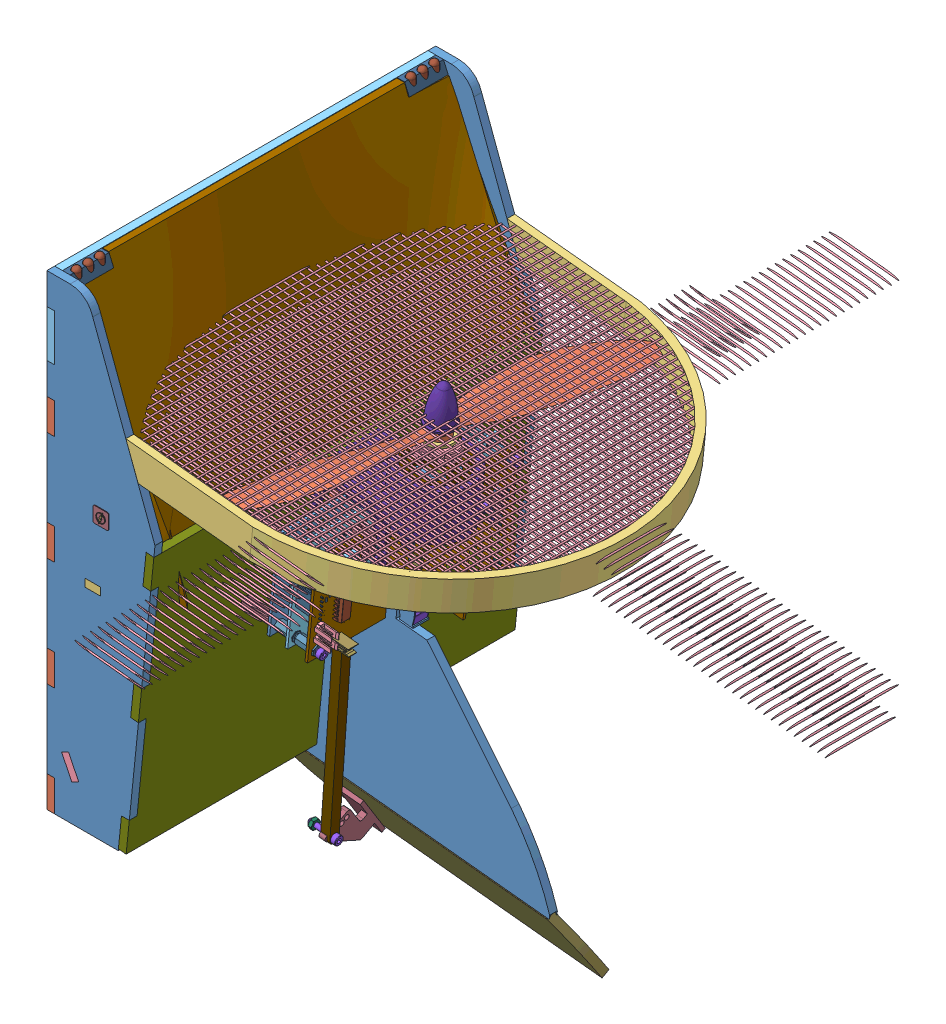
SolidWorks assembly AssTotaleSimu2, configuration Défaut. Lengths in mm.
Overall size (253.25 382.9 251.6).
1779 component instances, 238 part files, 11 mates.
Components (placement in the parent):
- AssStructSimu-1: AssStructSimu [Défaut] at (-125.7658 -1.8483 624.6548) x (1 0 0) z (0 0 -1) size (253.25 324.59 251.6)
  - AssBase-1: AssBase [Défaut] at (36.5482 -71.0398 34.0612) size (86.08 302.3 251.6)
    - AssD-1: AssD [Défaut] at (39.0992 31.0201 8.5) size (69.5 300 22)
      - P1-1: P1 [Défaut] at (-95.5819 194.6656 377.5) size (69.5 300 5)
      - P5-1: P5 [Défaut] at (-100.5819 -35.3344 360.5) x (0 1 0) z (1 0 0) size (230 22 5)
    - AssG-1: AssG [Défaut] at (39.0992 31.0201 -236.5) size (69.5 300 22)
      - P1-1: P1 [Défaut] at (-95.5819 194.6656 377.5) size (69.5 300 5)
      - P5-1: P5 [Défaut] at (-95.5819 -35.3344 399.5) x (0 1 0) z (-1 0 0) size (230 22 5)
    - P7-1: P7 [Défaut] at (-1.4828 89.6857 370.5) x (0 0 -1) z (0 -1 0) size (250 54.5 5)
    - P4-1: P4 [Défaut] at (-63.2363 165.9323 386) x (0 0 -1) z (0.898794 -0.438371 0) size (250 60.5 66.27)
    - P3-1: P3 [Défaut] at (-56.4828 -74.3143 146) x (0 0 1) z (-1 0 0) size (250 70 5)
    - P4b-1: P4b [Défaut] at (-58.7423 163.7404 190) x (0 0 1) z (0.438371 0.898794 0) size (152 56 2)
    - battery-1: battery [Défaut] at (-39.0156 204.1861 197.5) x (0 0 1) z (0.898794 -0.438371 0) size (137 43 30)
    - socket head cap screw 4762_din-1: socket head cap screw 4762_din [EN ISO 4762 M3 x 10 - 10N] at (-27.7008 145.2627 193) x (0.438371 0.898794 0) z (0 0 -1) size (13 5.5 5.5)
    - socket head cap screw 4762_din-2: socket head cap screw 4762_din [EN ISO 4762 M3 x 10 - 10N] at (-27.7008 145.2627 339) x (0.438371 0.898794 0) z (-0.791285 0.385936 -0.474259) size (13 5.5 5.5)
    - socket head cap screw 4762_din-3: socket head cap screw 4762_din [EN ISO 4762 M3 x 10 - 10N] at (-42.0815 152.2766 339) x (0.438371 0.898794 0) z (-0.001489 0.000726 -0.999999) size (13 5.5 5.5)
    - socket head cap screw 4762_din-4: socket head cap screw 4762_din [EN ISO 4762 M3 x 10 - 10N] at (-42.0815 152.2766 193) x (0.438371 0.898794 0) z (-0.031331 0.015281 -0.999392) size (13 5.5 5.5)
    - P11-1: P11 [Défaut] at (-57.5734 -73.9703 146.7843) x (0.005072 0 0.999987) z (0.006197 0.999981 -0.000031) size (240 65 164)
    - AssPhare-1: AssPhare [Défaut] at (-52.8518 -67.6977 411) x (0 1 0) z (0 0 -1) size (35.8 8 25)
      - piece_led-1: piece_led [Défaut] at (-6.6166 -3.631 25) size (7 8 25)
      - LED 5mm-1: LED 5mm [Valor predeterminado] at (-0.1166 0.369 30) x (0 0 1) z (-1 0 0) size (10.06 6 40.8)
      - LED 5mm-2: LED 5mm [Valor predeterminado] at (-0.1166 0.369 37.5) x (0 0 1) z (-1 0 0) size (10.06 6 40.8)
      - LED 5mm-3: LED 5mm [Valor predeterminado] at (-0.1166 0.369 45) x (0 0 1) z (-1 0 0) size (10.06 6 40.8)
    - AssPhare-2: AssPhare [Défaut] at (-52.8518 -67.6977 196) x (0 1 0) z (0 0 -1) size (35.8 8 25)
      - piece_led-1: piece_led [Défaut] at (-6.6166 -3.631 25) size (7 8 25)
      - LED 5mm-1: LED 5mm [Valor predeterminado] at (-0.1166 0.369 30) x (0 0 1) z (-1 0 0) size (10.06 6 40.8)
      - LED 5mm-2: LED 5mm [Valor predeterminado] at (-0.1166 0.369 37.5) x (0 0 1) z (-1 0 0) size (10.06 6 40.8)
      - LED 5mm-3: LED 5mm [Valor predeterminado] at (-0.1166 0.369 45) x (0 0 1) z (-1 0 0) size (10.06 6 40.8)
    - AssLogo-1: AssLogo [Défaut] at (-27.8835 45.1673 148.1054) x (-1 0 0) z (0 0 -1) size (10 10 0.8)
      - logo1-1: logo1 [Défaut] at (-6.5271 -4.4734 6.5054) size (5.8 7.71 0.4)
      - logo2-1: logo2 [Défaut] at (-6.4007 -4.4815 7.1054) size (10 10 0.4)
    - AssLogo-2: AssLogo [Défaut] at (-25.082 45.1673 383.8946) size (10 10 0.8)
      - logo1-1: logo1 [Défaut] at (-6.5271 -4.4734 6.5054) size (5.8 7.71 0.4)
      - logo2-1: logo2 [Défaut] at (-6.4007 -4.4815 7.1054) size (10 10 0.4)
    - support2-1: support2 [Défaut] at (-61.5648 191.7124 276) x (-0.017452 -0.999848 0) z (0.999848 -0.017452 0) size (75 20 10)
    - socket head cap screw 4762_din-5: socket head cap screw 4762_din [EN ISO 4762 M3 x 5 - 5N] at (-61.652 186.7132 269.3333) x (0.999848 -0.017452 0) z (-0.002158 -0.123615 0.992328) size (8 5.5 5.5)
    - socket head cap screw 4762_din-6: socket head cap screw 4762_din [EN ISO 4762 M3 x 5 - 5N] at (-61.652 186.7132 262.6667) x (0.999848 -0.017452 0) z (0 0 1) size (8 5.5 5.5)
    - socket head cap screw 4762_din-7: socket head cap screw 4762_din [EN ISO 4762 M3 x 25 - 18N] at (-55.2963 121.0922 253) x (0 0 1) z (-1 0 0) size (28 5.5 5.5)
    - hex nut style 1 gradeab_din-1: hex nut style 1 gradeab_din [Hexagon Nut ISO 4032 - M3 - W - N] at (-55.2963 121.0922 276) x (-0.923728 -0.383049 0) z (0 0 -1) size (5.5 6.35 2.4)
  - AssToitMot-1: AssToitMot [Défaut] at (-168.5238 43.6961 238.494) x (0 0 -1) z (0.9948 0.101852 0) size (250 207.5 205)
    - AssToit-1: AssToit [Défaut] at (-23.0702 -16.5789 -3.7148) size (250 207.5 205)
      - P8-1: P8 [Défaut] at (-38.4971 122.5921 203.5) size (250 175 5)
      - P12-1: P12 [Défaut] at (-60.4971 -63.4079 265.5) x (1 0 0) z (0 -1 0) size (44.28 76.64 55)
      - P13-1: P13 [Défaut] at (-35.9971 -52.8579 208.5) x (0 0 1) z (-1 0 0) size (64 15.55 5)
      - P10_2-1: P10_2 [Défaut] at (-35.9971 111.5921 171) x (0 0 1) z (-1 0 0) size (188.5 117.6 5)
    - Parallax-Servo_DUMMY-1: Parallax-Servo_DUMMY [Défaut] at (-61.6002 -51.5207 216.6662) x (1 0 0) z (0 1 0) size (20.07 42.67 55.64)
    - socket head cap screw 4762_din-1: socket head cap screw 4762_din [EN ISO 4762 M2.5 x 5 - 5N] at (-51.9272 -76.4868 259.2852) x (0 -1 0) z (-0.546944 0 0.837169) size (7.5 4.5 4.5)
    - socket head cap screw 4762_din-2: socket head cap screw 4762_din [EN ISO 4762 M2.5 x 5 - 5N] at (-61.5672 -76.4868 268.9252) x (0 -1 0) z (-0.546944 0 0.837169) size (7.5 4.5 4.5)
    - socket head cap screw 4762_din-3: socket head cap screw 4762_din [EN ISO 4762 M2.5 x 5 - 5N] at (-71.2072 -76.4868 259.2852) x (0 -1 0) z (-0.546944 0 0.837169) size (7.5 4.5 4.5)
    - socket head cap screw 4762_din-4: socket head cap screw 4762_din [EN ISO 4762 M2.5 x 5 - 5N] at (-61.5672 -76.4868 249.6452) x (0 -1 0) z (-0.546944 0 0.837169) size (7.5 4.5 4.5)
    - AssPhare-1: AssPhare [Défaut] at (8.4328 83.3966 196.1542) x (0 -1 0) z (1 0 0) size (35.8 8 25)
      - piece_led-1: piece_led [Défaut] at (-6.6166 -3.631 25) size (7 8 25)
      - LED 5mm-1: LED 5mm [Valor predeterminado] at (-0.1166 0.369 30) x (0 0 1) z (-1 0 0) size (10.06 6 40.8)
      - LED 5mm-2: LED 5mm [Valor predeterminado] at (-0.1166 0.369 37.5) x (0 0 1) z (-1 0 0) size (10.06 6 40.8)
      - LED 5mm-3: LED 5mm [Valor predeterminado] at (-0.1166 0.369 45) x (0 0 1) z (-1 0 0) size (10.06 6 40.8)
    - AssPhare-2: AssPhare [Défaut] at (-206.5672 83.3966 196.1542) x (0 -1 0) z (1 0 0) size (35.8 8 25)
      - piece_led-1: piece_led [Défaut] at (-6.6166 -3.631 25) size (7 8 25)
      - LED 5mm-1: LED 5mm [Valor predeterminado] at (-0.1166 0.369 30) x (0 0 1) z (-1 0 0) size (10.06 6 40.8)
      - LED 5mm-2: LED 5mm [Valor predeterminado] at (-0.1166 0.369 37.5) x (0 0 1) z (-1 0 0) size (10.06 6 40.8)
      - LED 5mm-3: LED 5mm [Valor predeterminado] at (-0.1166 0.369 45) x (0 0 1) z (-1 0 0) size (10.06 6 40.8)
    - socket head cap screw 4762_din-5: socket head cap screw 4762_din [EN ISO 4762 M3 x 10 - 10N] at (-67.0672 -22.9368 210.2852) x (0 0 -1) z (1 0 0) size (13 5.5 5.5)
    - socket head cap screw 4762_din-6: socket head cap screw 4762_din [EN ISO 4762 M3 x 10 - 10N] at (-56.0672 -72.9868 210.2852) x (0 0 -1) z (1 0 0) size (13 5.5 5.5)
    - socket head cap screw 4762_din-7: socket head cap screw 4762_din [EN ISO 4762 M3 x 10 - 10N] at (-67.0672 -72.9868 210.2852) x (0 0 -1) z (1 0 0) size (13 5.5 5.5)
    - socket head cap screw 4762_din-8: socket head cap screw 4762_din [EN ISO 4762 M3 x 10 - 10N] at (-56.0672 -22.9368 210.2852) x (0 0 -1) z (1 0 0) size (13 5.5 5.5)
    - hex nut style 1 gradeab_din-1: hex nut style 1 gradeab_din [Hexagon Nut ISO 4032 - M3 - W - N] at (-67.0672 -72.9868 197.3852) x (-0.923728 -0.383049 0) z (0 0 -1) size (5.5 6.35 2.4)
    - hex nut style 1 gradeab_din-2: hex nut style 1 gradeab_din [Hexagon Nut ISO 4032 - M3 - W - N] at (-56.0672 -72.9868 199.7852) size (5.5 6.35 2.4)
    - hex nut style 1 gradeab_din-3: hex nut style 1 gradeab_din [Hexagon Nut ISO 4032 - M3 - W - N] at (-67.0672 -22.9368 199.7852) size (5.5 6.35 2.4)
    - hex nut style 1 gradeab_din-4: hex nut style 1 gradeab_din [Hexagon Nut ISO 4032 - M3 - W - N] at (-56.0672 -22.9368 199.7852) size (5.5 6.35 2.4)
  - AssProtec-1: AssProtec [Défaut] at (86.6746 190.4649 284.6351) x (0 0 -1) z (0.101852 -0.9948 0) size (250 237.46 20)
    - protec3c-1: protec3c [Défaut] at (-140.4261 -87.7568 240) size (250 197 20)
    - AssGrillage-1: AssGrillage [Défaut] at (-370.4609 -132.5428 258.3161) x (0 0 -1) z (1 0 0) size (2.02 237.05 250)
      - barreau-1: barreau [Défaut] at (-1.1839 0.254 200) size (1 1 400)
      - barreau-3: barreau [Défaut] at (-1.1839 5.254 200) size (1 1 400)
      - barreau-4: barreau [Défaut] at (-1.1839 10.254 200) size (1 1 400)
      - barreau-5: barreau [Défaut] at (-1.1839 15.254 200) size (1 1 400)
      - barreau-6: barreau [Défaut] at (-1.1839 20.254 200) size (1 1 400)
      - barreau-7: barreau [Défaut] at (-1.1839 25.254 200) size (1 1 400)
      - barreau-8: barreau [Défaut] at (-1.1839 30.254 200) size (1 1 400)
      - barreau-9: barreau [Défaut] at (-1.1839 35.254 200) size (1 1 400)
      - barreau-10: barreau [Défaut] at (-1.1839 40.254 200) size (1 1 400)
      - barreau-11: barreau [Défaut] at (-1.1839 45.254 200) size (1 1 400)
      - barreau-12: barreau [Défaut] at (-1.1839 50.254 200) size (1 1 400)
      - barreau-13: barreau [Défaut] at (-1.1839 55.254 200) size (1 1 400)
      - barreau-14: barreau [Défaut] at (-1.1839 60.254 200) size (1 1 400)
      - barreau-15: barreau [Défaut] at (-1.1839 65.254 200) size (1 1 400)
      - barreau-16: barreau [Défaut] at (-1.1839 70.254 200) size (1 1 400)
      - barreau-17: barreau [Défaut] at (-1.1839 75.254 200) size (1 1 400)
      - barreau-18: barreau [Défaut] at (-1.1839 80.254 200) size (1 1 400)
      - barreau-19: barreau [Défaut] at (-1.1839 85.254 200) size (1 1 400)
      - barreau-20: barreau [Défaut] at (-1.1839 90.254 200) size (1 1 400)
      - barreau-21: barreau [Défaut] at (-1.1839 95.254 200) size (1 1 400)
      - barreau-22: barreau [Défaut] at (-1.1839 100.254 200) size (1 1 400)
      - barreau-23: barreau [Défaut] at (-1.1839 105.254 200) size (1 1 400)
      - barreau-24: barreau [Défaut] at (-1.1839 110.254 200) size (1 1 400)
      - barreau-25: barreau [Défaut] at (-1.1839 115.254 200) size (1 1 400)
      - barreau-26: barreau [Défaut] at (-1.1839 120.254 200) size (1 1 400)
      - barreau-27: barreau [Défaut] at (-1.1839 125.254 200) size (1 1 400)
      - barreau-28: barreau [Défaut] at (-1.1839 130.254 200) size (1 1 400)
      - barreau-29: barreau [Défaut] at (-1.1839 135.254 200) size (1 1 400)
      - barreau-30: barreau [Défaut] at (-1.1839 140.254 200) size (1 1 400)
      - barreau-31: barreau [Défaut] at (-1.1839 145.254 200) size (1 1 400)
      - barreau-32: barreau [Défaut] at (-1.1839 150.254 200) size (1 1 400)
      - barreau-33: barreau [Défaut] at (-1.1839 155.254 200) size (1 1 400)
      - barreau-34: barreau [Défaut] at (-1.1839 160.254 200) size (1 1 400)
      - barreau-35: barreau [Défaut] at (-1.1839 165.254 200) size (1 1 400)
      - barreau-36: barreau [Défaut] at (-1.1839 170.254 200) size (1 1 400)
      - barreau-37: barreau [Défaut] at (-1.1839 175.254 200) size (1 1 400)
      - barreau-38: barreau [Défaut] at (-1.1839 180.254 200) size (1 1 400)
      - barreau-39: barreau [Défaut] at (-1.1839 185.254 200) size (1 1 400)
      - barreau-40: barreau [Défaut] at (-1.1839 190.254 200) size (1 1 400)
      - barreau-41: barreau [Défaut] at (-1.1839 195.254 200) size (1 1 400)
      - barreau-42: barreau [Défaut] at (-0.1839 -1.5314 598.7823) x (0.998922 0 0.04641) z (0 1 0) size (1 1 400)
      - barreau-43: barreau [Défaut] at (-1.1839 200.254 200) size (1 1 400)
      - barreau-44: barreau [Défaut] at (-1.1839 205.254 200) size (1 1 400)
      - barreau-45: barreau [Défaut] at (-1.1839 210.254 200) size (1 1 400)
      - barreau-46: barreau [Défaut] at (-1.1839 215.254 200) size (1 1 400)
      - barreau-47: barreau [Défaut] at (-1.1839 220.254 200) size (1 1 400)
      - barreau-48: barreau [Défaut] at (-1.1839 225.254 200) size (1 1 400)
      - barreau-49: barreau [Défaut] at (-1.1839 230.254 200) size (1 1 400)
      - barreau-50: barreau [Défaut] at (-1.1839 235.254 200) size (1 1 400)
      - barreau-51: barreau [Défaut] at (-1.1839 240.254 200) size (1 1 400)
      - barreau-52: barreau [Défaut] at (-1.1839 245.254 200) size (1 1 400)
      - barreau-53: barreau [Défaut] at (-1.1839 250.254 200) size (1 1 400)
      - barreau-54: barreau [Défaut] at (-1.1839 255.254 200) size (1 1 400)
      - barreau-55: barreau [Défaut] at (-1.1839 260.254 200) size (1 1 400)
      - barreau-56: barreau [Défaut] at (-1.1839 265.254 200) size (1 1 400)
      - barreau-57: barreau [Défaut] at (-1.1839 270.254 200) size (1 1 400)
      - barreau-58: barreau [Défaut] at (-1.1839 275.254 200) size (1 1 400)
      - barreau-59: barreau [Défaut] at (-1.1839 280.254 200) size (1 1 400)
      - barreau-60: barreau [Défaut] at (-1.1839 285.254 200) size (1 1 400)
      - barreau-61: barreau [Défaut] at (-1.1839 290.254 200) size (1 1 400)
      - barreau-62: barreau [Défaut] at (-1.1839 295.254 200) size (1 1 400)
      - barreau-63: barreau [Défaut] at (-1.1839 300.254 200) size (1 1 400)
      - barreau-64: barreau [Défaut] at (-1.1839 305.254 200) size (1 1 400)
      - barreau-65: barreau [Défaut] at (-1.1839 310.254 200) size (1 1 400)
      - barreau-66: barreau [Défaut] at (-1.1839 315.254 200) size (1 1 400)
      - barreau-67: barreau [Défaut] at (-1.1839 320.254 200) size (1 1 400)
      - barreau-68: barreau [Défaut] at (-1.1839 325.254 200) size (1 1 400)
      - barreau-69: barreau [Défaut] at (-1.1839 330.254 200) size (1 1 400)
      - barreau-70: barreau [Défaut] at (-1.1839 335.254 200) size (1 1 400)
      - barreau-71: barreau [Défaut] at (-1.1839 340.254 200) size (1 1 400)
      - barreau-72: barreau [Défaut] at (-1.1839 345.254 200) size (1 1 400)
      - barreau-73: barreau [Défaut] at (-1.1839 350.254 200) size (1 1 400)
      - barreau-74: barreau [Défaut] at (-1.1839 355.254 200) size (1 1 400)
      - barreau-75: barreau [Défaut] at (-1.1839 360.254 200) size (1 1 400)
      - barreau-76: barreau [Défaut] at (-1.1839 365.254 200) size (1 1 400)
      - barreau-77: barreau [Défaut] at (-1.1839 370.254 200) size (1 1 400)
      - barreau-78: barreau [Défaut] at (-1.1839 375.254 200) size (1 1 400)
      - barreau-79: barreau [Défaut] at (-1.1839 380.254 200) size (1 1 400)
      - barreau-80: barreau [Défaut] at (-1.1839 385.254 200) size (1 1 400)
      - barreau-81: barreau [Défaut] at (-1.1839 390.254 200) size (1 1 400)
      - barreau-82: barreau [Défaut] at (-1.1839 395.254 200) size (1 1 400)
      - barreau-136: barreau [Défaut] at (-0.1839 -1.5314 593.7823) x (0.998922 0 0.04641) z (0 1 0) size (1 1 400)
      - barreau-137: barreau [Défaut] at (-0.1839 -1.5314 588.7823) x (0.998922 0 0.04641) z (0 1 0) size (1 1 400)
      - barreau-138: barreau [Défaut] at (-0.1839 -1.5314 583.7823) x (0.998922 0 0.04641) z (0 1 0) size (1 1 400)
      - barreau-139: barreau [Défaut] at (-0.1839 -1.5314 578.7823) x (0.998922 0 0.04641) z (0 1 0) size (1 1 400)
      - barreau-140: barreau [Défaut] at (-0.1839 -1.5314 573.7823) x (0.998922 0 0.04641) z (0 1 0) size (1 1 400)
      - barreau-141: barreau [Défaut] at (-0.1839 -1.5314 568.7823) x (0.998922 0 0.04641) z (0 1 0) size (1 1 400)
      - barreau-142: barreau [Défaut] at (-0.1839 -1.5314 563.7823) x (0.998922 0 0.04641) z (0 1 0) size (1 1 400)
      - barreau-143: barreau [Défaut] at (-0.1839 -1.5314 558.7823) x (0.998922 0 0.04641) z (0 1 0) size (1 1 400)
      - barreau-144: barreau [Défaut] at (-0.1839 -1.5314 553.7823) x (0.998922 0 0.04641) z (0 1 0) size (1 1 400)
      - barreau-145: barreau [Défaut] at (-0.1839 -1.5314 548.7823) x (0.998922 0 0.04641) z (0 1 0) size (1 1 400)
      - barreau-146: barreau [Défaut] at (-0.1839 -1.5314 543.7823) x (0.998922 0 0.04641) z (0 1 0) size (1 1 400)
      - barreau-147: barreau [Défaut] at (-0.1839 -1.5314 538.7823) x (0.998922 0 0.04641) z (0 1 0) size (1 1 400)
      - barreau-148: barreau [Défaut] at (-0.1839 -1.5314 533.7823) x (0.998922 0 0.04641) z (0 1 0) size (1 1 400)
      - barreau-149: barreau [Défaut] at (-0.1839 -1.5314 528.7823) x (0.998922 0 0.04641) z (0 1 0) size (1 1 400)
      - barreau-150: barreau [Défaut] at (-0.1839 -1.5314 523.7823) x (0.998922 0 0.04641) z (0 1 0) size (1 1 400)
      - barreau-151: barreau [Défaut] at (-0.1839 -1.5314 518.7823) x (0.998922 0 0.04641) z (0 1 0) size (1 1 400)
      - barreau-152: barreau [Défaut] at (-0.1839 -1.5314 513.7823) x (0.998922 0 0.04641) z (0 1 0) size (1 1 400)
      - barreau-153: barreau [Défaut] at (-0.1839 -1.5314 508.7823) x (0.998922 0 0.04641) z (0 1 0) size (1 1 400)
      - barreau-154: barreau [Défaut] at (-0.1839 -1.5314 503.7823) x (0.998922 0 0.04641) z (0 1 0) size (1 1 400)
      - barreau-155: barreau [Défaut] at (-0.1839 -1.5314 498.7823) x (0.998922 0 0.04641) z (0 1 0) size (1 1 400)
      - barreau-156: barreau [Défaut] at (-0.1839 -1.5314 493.7823) x (0.998922 0 0.04641) z (0 1 0) size (1 1 400)
      - barreau-157: barreau [Défaut] at (-0.1839 -1.5314 488.7823) x (0.998922 0 0.04641) z (0 1 0) size (1 1 400)
      - barreau-158: barreau [Défaut] at (-0.1839 -1.5314 483.7823) x (0.998922 0 0.04641) z (0 1 0) size (1 1 400)
      - barreau-159: barreau [Défaut] at (-0.1839 -1.5314 478.7823) x (0.998922 0 0.04641) z (0 1 0) size (1 1 400)
      - barreau-160: barreau [Défaut] at (-0.1839 -1.5314 473.7823) x (0.998922 0 0.04641) z (0 1 0) size (1 1 400)
      - barreau-161: barreau [Défaut] at (-0.1839 -1.5314 468.7823) x (0.998922 0 0.04641) z (0 1 0) size (1 1 400)
      - barreau-162: barreau [Défaut] at (-0.1839 -1.5314 463.7823) x (0.998922 0 0.04641) z (0 1 0) size (1 1 400)
      - barreau-163: barreau [Défaut] at (-0.1839 -1.5314 458.7823) x (0.998922 0 0.04641) z (0 1 0) size (1 1 400)
      - barreau-164: barreau [Défaut] at (-0.1839 -1.5314 453.7823) x (0.998922 0 0.04641) z (0 1 0) size (1 1 400)
      - barreau-165: barreau [Défaut] at (-0.1839 -1.5314 448.7823) x (0.998922 0 0.04641) z (0 1 0) size (1 1 400)
      - barreau-166: barreau [Défaut] at (-0.1839 -1.5314 443.7823) x (0.998922 0 0.04641) z (0 1 0) size (1 1 400)
      - barreau-167: barreau [Défaut] at (-0.1839 -1.5314 438.7823) x (0.998922 0 0.04641) z (0 1 0) size (1 1 400)
      - barreau-168: barreau [Défaut] at (-0.1839 -1.5314 433.7823) x (0.998922 0 0.04641) z (0 1 0) size (1 1 400)
      - barreau-169: barreau [Défaut] at (-0.1839 -1.5314 428.7823) x (0.998922 0 0.04641) z (0 1 0) size (1 1 400)
      - barreau-170: barreau [Défaut] at (-0.1839 -1.5314 423.7823) x (0.998922 0 0.04641) z (0 1 0) size (1 1 400)
      - barreau-171: barreau [Défaut] at (-0.1839 -1.5314 418.7823) x (0.998922 0 0.04641) z (0 1 0) size (1 1 400)
      - barreau-172: barreau [Défaut] at (-0.1839 -1.5314 413.7823) x (0.998922 0 0.04641) z (0 1 0) size (1 1 400)
      - barreau-173: barreau [Défaut] at (-0.1839 -1.5314 408.7823) x (0.998922 0 0.04641) z (0 1 0) size (1 1 400)
      - barreau-174: barreau [Défaut] at (-0.1839 -1.5314 403.7823) x (0.998922 0 0.04641) z (0 1 0) size (1 1 400)
      - barreau-175: barreau [Défaut] at (-0.1839 -1.5314 398.7823) x (0.998922 0 0.04641) z (0 1 0) size (1 1 400)
      - barreau-176: barreau [Défaut] at (-0.1839 -1.5314 393.7823) x (0.998922 0 0.04641) z (0 1 0) size (1 1 400)
      - barreau-177: barreau [Défaut] at (-0.1839 -1.5314 388.7823) x (0.998922 0 0.04641) z (0 1 0) size (1 1 400)
      - barreau-178: barreau [Défaut] at (-0.1839 -1.5314 383.7823) x (0.998922 0 0.04641) z (0 1 0) size (1 1 400)
      - barreau-179: barreau [Défaut] at (-0.1839 -1.5314 378.7823) x (0.998922 0 0.04641) z (0 1 0) size (1 1 400)
      - barreau-180: barreau [Défaut] at (-0.1839 -1.5314 373.7823) x (0.998922 0 0.04641) z (0 1 0) size (1 1 400)
      - barreau-181: barreau [Défaut] at (-0.1839 -1.5314 368.7823) x (0.998922 0 0.04641) z (0 1 0) size (1 1 400)
      - barreau-182: barreau [Défaut] at (-0.1839 -1.5314 363.7823) x (0.998922 0 0.04641) z (0 1 0) size (1 1 400)
      - barreau-183: barreau [Défaut] at (-0.1839 -1.5314 358.7823) x (0.998922 0 0.04641) z (0 1 0) size (1 1 400)
      - barreau-184: barreau [Défaut] at (-0.1839 -1.5314 353.7823) x (0.998922 0 0.04641) z (0 1 0) size (1 1 400)
      - barreau-185: barreau [Défaut] at (-0.1839 -1.5314 348.7823) x (0.998922 0 0.04641) z (0 1 0) size (1 1 400)
      - barreau-186: barreau [Défaut] at (-0.1839 -1.5314 343.7823) x (0.998922 0 0.04641) z (0 1 0) size (1 1 400)
      - barreau-187: barreau [Défaut] at (-0.1839 -1.5314 338.7823) x (0.998922 0 0.04641) z (0 1 0) size (1 1 400)
      - barreau-188: barreau [Défaut] at (-0.1839 -1.5314 333.7823) x (0.998922 0 0.04641) z (0 1 0) size (1 1 400)
      - barreau-189: barreau [Défaut] at (-0.1839 -1.5314 328.7823) x (0.998922 0 0.04641) z (0 1 0) size (1 1 400)
      - barreau-190: barreau [Défaut] at (-0.1839 -1.5314 323.7823) x (0.998922 0 0.04641) z (0 1 0) size (1 1 400)
      - barreau-191: barreau [Défaut] at (-0.1839 -1.5314 318.7823) x (0.998922 0 0.04641) z (0 1 0) size (1 1 400)
      - barreau-192: barreau [Défaut] at (-0.1839 -1.5314 313.7823) x (0.998922 0 0.04641) z (0 1 0) size (1 1 400)
      - barreau-193: barreau [Défaut] at (-0.1839 -1.5314 308.7823) x (0.998922 0 0.04641) z (0 1 0) size (1 1 400)
      - barreau-194: barreau [Défaut] at (-0.1839 -1.5314 303.7823) x (0.998922 0 0.04641) z (0 1 0) size (1 1 400)
      - barreau-195: barreau [Défaut] at (-0.1839 -1.5314 298.7823) x (0.998922 0 0.04641) z (0 1 0) size (1 1 400)
      - barreau-196: barreau [Défaut] at (-0.1839 -1.5314 293.7823) x (0.998922 0 0.04641) z (0 1 0) size (1 1 400)
      - barreau-197: barreau [Défaut] at (-0.1839 -1.5314 288.7823) x (0.998922 0 0.04641) z (0 1 0) size (1 1 400)
      - barreau-198: barreau [Défaut] at (-0.1839 -1.5314 283.7823) x (0.998922 0 0.04641) z (0 1 0) size (1 1 400)
      - barreau-199: barreau [Défaut] at (-0.1839 -1.5314 278.7823) x (0.998922 0 0.04641) z (0 1 0) size (1 1 400)
      - barreau-200: barreau [Défaut] at (-0.1839 -1.5314 273.7823) x (0.998922 0 0.04641) z (0 1 0) size (1 1 400)
      - barreau-201: barreau [Défaut] at (-0.1839 -1.5314 268.7823) x (0.998922 0 0.04641) z (0 1 0) size (1 1 400)
      - barreau-202: barreau [Défaut] at (-0.1839 -1.5314 263.7823) x (0.998922 0 0.04641) z (0 1 0) size (1 1 400)
      - barreau-203: barreau [Défaut] at (-0.1839 -1.5314 258.7823) x (0.998922 0 0.04641) z (0 1 0) size (1 1 400)
      - barreau-204: barreau [Défaut] at (-0.1839 -1.5314 253.7823) x (0.998922 0 0.04641) z (0 1 0) size (1 1 400)
      - barreau-205: barreau [Défaut] at (-0.1839 -1.5314 248.7823) x (0.998922 0 0.04641) z (0 1 0) size (1 1 400)
      - barreau-206: barreau [Défaut] at (-0.1839 -1.5314 243.7823) x (0.998922 0 0.04641) z (0 1 0) size (1 1 400)
      - barreau-207: barreau [Défaut] at (-0.1839 -1.5314 238.7823) x (0.998922 0 0.04641) z (0 1 0) size (1 1 400)
      - barreau-208: barreau [Défaut] at (-0.1839 -1.5314 233.7823) x (0.998922 0 0.04641) z (0 1 0) size (1 1 400)
      - barreau-209: barreau [Défaut] at (-0.1839 -1.5314 228.7823) x (0.998922 0 0.04641) z (0 1 0) size (1 1 400)
      - barreau-210: barreau [Défaut] at (-0.1839 -1.5314 223.7823) x (0.998922 0 0.04641) z (0 1 0) size (1 1 400)
      - barreau-211: barreau [Défaut] at (-0.1839 -1.5314 218.7823) x (0.998922 0 0.04641) z (0 1 0) size (1 1 400)
      - barreau-212: barreau [Défaut] at (-0.1839 -1.5314 213.7823) x (0.998922 0 0.04641) z (0 1 0) size (1 1 400)
      - barreau-213: barreau [Défaut] at (-0.1839 -1.5314 208.7823) x (0.998922 0 0.04641) z (0 1 0) size (1 1 400)
      - barreau-214: barreau [Défaut] at (-0.1839 -1.5314 203.7823) x (0.998922 0 0.04641) z (0 1 0) size (1 1 400)
    - AssGrillage-2: AssGrillage [Défaut] at (339.6086 -132.5428 241.6839) x (0 0 1) z (-1 0 0) size (2.02 237.05 250)
      - barreau-1: barreau [Défaut] at (-1.1839 0.254 200) size (1 1 400)
      - barreau-3: barreau [Défaut] at (-1.1839 5.254 200) size (1 1 400)
      - barreau-4: barreau [Défaut] at (-1.1839 10.254 200) size (1 1 400)
      - barreau-5: barreau [Défaut] at (-1.1839 15.254 200) size (1 1 400)
      - barreau-6: barreau [Défaut] at (-1.1839 20.254 200) size (1 1 400)
      - barreau-7: barreau [Défaut] at (-1.1839 25.254 200) size (1 1 400)
      - barreau-8: barreau [Défaut] at (-1.1839 30.254 200) size (1 1 400)
      - barreau-9: barreau [Défaut] at (-1.1839 35.254 200) size (1 1 400)
      - barreau-10: barreau [Défaut] at (-1.1839 40.254 200) size (1 1 400)
      - barreau-11: barreau [Défaut] at (-1.1839 45.254 200) size (1 1 400)
      - barreau-12: barreau [Défaut] at (-1.1839 50.254 200) size (1 1 400)
      - barreau-13: barreau [Défaut] at (-1.1839 55.254 200) size (1 1 400)
      - barreau-14: barreau [Défaut] at (-1.1839 60.254 200) size (1 1 400)
      - barreau-15: barreau [Défaut] at (-1.1839 65.254 200) size (1 1 400)
      - barreau-16: barreau [Défaut] at (-1.1839 70.254 200) size (1 1 400)
      - barreau-17: barreau [Défaut] at (-1.1839 75.254 200) size (1 1 400)
      - barreau-18: barreau [Défaut] at (-1.1839 80.254 200) size (1 1 400)
      - barreau-19: barreau [Défaut] at (-1.1839 85.254 200) size (1 1 400)
      - barreau-20: barreau [Défaut] at (-1.1839 90.254 200) size (1 1 400)
      - barreau-21: barreau [Défaut] at (-1.1839 95.254 200) size (1 1 400)
      - barreau-22: barreau [Défaut] at (-1.1839 100.254 200) size (1 1 400)
      - barreau-23: barreau [Défaut] at (-1.1839 105.254 200) size (1 1 400)
      - barreau-24: barreau [Défaut] at (-1.1839 110.254 200) size (1 1 400)
      - barreau-25: barreau [Défaut] at (-1.1839 115.254 200) size (1 1 400)
      - barreau-26: barreau [Défaut] at (-1.1839 120.254 200) size (1 1 400)
      - barreau-27: barreau [Défaut] at (-1.1839 125.254 200) size (1 1 400)
      - barreau-28: barreau [Défaut] at (-1.1839 130.254 200) size (1 1 400)
      - barreau-29: barreau [Défaut] at (-1.1839 135.254 200) size (1 1 400)
      - barreau-30: barreau [Défaut] at (-1.1839 140.254 200) size (1 1 400)
      - barreau-31: barreau [Défaut] at (-1.1839 145.254 200) size (1 1 400)
      - barreau-32: barreau [Défaut] at (-1.1839 150.254 200) size (1 1 400)
      - barreau-33: barreau [Défaut] at (-1.1839 155.254 200) size (1 1 400)
      - barreau-34: barreau [Défaut] at (-1.1839 160.254 200) size (1 1 400)
      - barreau-35: barreau [Défaut] at (-1.1839 165.254 200) size (1 1 400)
      - barreau-36: barreau [Défaut] at (-1.1839 170.254 200) size (1 1 400)
      - barreau-37: barreau [Défaut] at (-1.1839 175.254 200) size (1 1 400)
      - barreau-38: barreau [Défaut] at (-1.1839 180.254 200) size (1 1 400)
      - barreau-39: barreau [Défaut] at (-1.1839 185.254 200) size (1 1 400)
      - barreau-40: barreau [Défaut] at (-1.1839 190.254 200) size (1 1 400)
      - barreau-41: barreau [Défaut] at (-1.1839 195.254 200) size (1 1 400)
      - barreau-42: barreau [Défaut] at (-0.1839 -1.5314 598.7823) x (0.998922 0 0.04641) z (0 1 0) size (1 1 400)
      - barreau-43: barreau [Défaut] at (-1.1839 200.254 200) size (1 1 400)
      - barreau-44: barreau [Défaut] at (-1.1839 205.254 200) size (1 1 400)
      - barreau-45: barreau [Défaut] at (-1.1839 210.254 200) size (1 1 400)
      - barreau-46: barreau [Défaut] at (-1.1839 215.254 200) size (1 1 400)
      - barreau-47: barreau [Défaut] at (-1.1839 220.254 200) size (1 1 400)
      - barreau-48: barreau [Défaut] at (-1.1839 225.254 200) size (1 1 400)
      - barreau-49: barreau [Défaut] at (-1.1839 230.254 200) size (1 1 400)
      - barreau-50: barreau [Défaut] at (-1.1839 235.254 200) size (1 1 400)
      - barreau-51: barreau [Défaut] at (-1.1839 240.254 200) size (1 1 400)
      - barreau-52: barreau [Défaut] at (-1.1839 245.254 200) size (1 1 400)
      - barreau-53: barreau [Défaut] at (-1.1839 250.254 200) size (1 1 400)
      - barreau-54: barreau [Défaut] at (-1.1839 255.254 200) size (1 1 400)
      - barreau-55: barreau [Défaut] at (-1.1839 260.254 200) size (1 1 400)
      - barreau-56: barreau [Défaut] at (-1.1839 265.254 200) size (1 1 400)
      - barreau-57: barreau [Défaut] at (-1.1839 270.254 200) size (1 1 400)
      - barreau-58: barreau [Défaut] at (-1.1839 275.254 200) size (1 1 400)
      - barreau-59: barreau [Défaut] at (-1.1839 280.254 200) size (1 1 400)
      - barreau-60: barreau [Défaut] at (-1.1839 285.254 200) size (1 1 400)
      - barreau-61: barreau [Défaut] at (-1.1839 290.254 200) size (1 1 400)
      - barreau-62: barreau [Défaut] at (-1.1839 295.254 200) size (1 1 400)
      - barreau-63: barreau [Défaut] at (-1.1839 300.254 200) size (1 1 400)
      - barreau-64: barreau [Défaut] at (-1.1839 305.254 200) size (1 1 400)
      - barreau-65: barreau [Défaut] at (-1.1839 310.254 200) size (1 1 400)
      - barreau-66: barreau [Défaut] at (-1.1839 315.254 200) size (1 1 400)
      - barreau-67: barreau [Défaut] at (-1.1839 320.254 200) size (1 1 400)
      - barreau-68: barreau [Défaut] at (-1.1839 325.254 200) size (1 1 400)
      - barreau-69: barreau [Défaut] at (-1.1839 330.254 200) size (1 1 400)
      - barreau-70: barreau [Défaut] at (-1.1839 335.254 200) size (1 1 400)
      - barreau-71: barreau [Défaut] at (-1.1839 340.254 200) size (1 1 400)
      - barreau-72: barreau [Défaut] at (-1.1839 345.254 200) size (1 1 400)
      - barreau-73: barreau [Défaut] at (-1.1839 350.254 200) size (1 1 400)
      - barreau-74: barreau [Défaut] at (-1.1839 355.254 200) size (1 1 400)
      - barreau-75: barreau [Défaut] at (-1.1839 360.254 200) size (1 1 400)
      - barreau-76: barreau [Défaut] at (-1.1839 365.254 200) size (1 1 400)
      - barreau-77: barreau [Défaut] at (-1.1839 370.254 200) size (1 1 400)
      - barreau-78: barreau [Défaut] at (-1.1839 375.254 200) size (1 1 400)
      - barreau-79: barreau [Défaut] at (-1.1839 380.254 200) size (1 1 400)
      - barreau-80: barreau [Défaut] at (-1.1839 385.254 200) size (1 1 400)
      - barreau-81: barreau [Défaut] at (-1.1839 390.254 200) size (1 1 400)
      - barreau-82: barreau [Défaut] at (-1.1839 395.254 200) size (1 1 400)
      - barreau-136: barreau [Défaut] at (-0.1839 -1.5314 593.7823) x (0.998922 0 0.04641) z (0 1 0) size (1 1 400)
      - barreau-137: barreau [Défaut] at (-0.1839 -1.5314 588.7823) x (0.998922 0 0.04641) z (0 1 0) size (1 1 400)
      - barreau-138: barreau [Défaut] at (-0.1839 -1.5314 583.7823) x (0.998922 0 0.04641) z (0 1 0) size (1 1 400)
      - barreau-139: barreau [Défaut] at (-0.1839 -1.5314 578.7823) x (0.998922 0 0.04641) z (0 1 0) size (1 1 400)
      - barreau-140: barreau [Défaut] at (-0.1839 -1.5314 573.7823) x (0.998922 0 0.04641) z (0 1 0) size (1 1 400)
      - barreau-141: barreau [Défaut] at (-0.1839 -1.5314 568.7823) x (0.998922 0 0.04641) z (0 1 0) size (1 1 400)
      - barreau-142: barreau [Défaut] at (-0.1839 -1.5314 563.7823) x (0.998922 0 0.04641) z (0 1 0) size (1 1 400)
      - barreau-143: barreau [Défaut] at (-0.1839 -1.5314 558.7823) x (0.998922 0 0.04641) z (0 1 0) size (1 1 400)
      - barreau-144: barreau [Défaut] at (-0.1839 -1.5314 553.7823) x (0.998922 0 0.04641) z (0 1 0) size (1 1 400)
      - barreau-145: barreau [Défaut] at (-0.1839 -1.5314 548.7823) x (0.998922 0 0.04641) z (0 1 0) size (1 1 400)
      - barreau-146: barreau [Défaut] at (-0.1839 -1.5314 543.7823) x (0.998922 0 0.04641) z (0 1 0) size (1 1 400)
      - barreau-147: barreau [Défaut] at (-0.1839 -1.5314 538.7823) x (0.998922 0 0.04641) z (0 1 0) size (1 1 400)
      - barreau-148: barreau [Défaut] at (-0.1839 -1.5314 533.7823) x (0.998922 0 0.04641) z (0 1 0) size (1 1 400)
      - barreau-149: barreau [Défaut] at (-0.1839 -1.5314 528.7823) x (0.998922 0 0.04641) z (0 1 0) size (1 1 400)
      - barreau-150: barreau [Défaut] at (-0.1839 -1.5314 523.7823) x (0.998922 0 0.04641) z (0 1 0) size (1 1 400)
      - barreau-151: barreau [Défaut] at (-0.1839 -1.5314 518.7823) x (0.998922 0 0.04641) z (0 1 0) size (1 1 400)
      - barreau-152: barreau [Défaut] at (-0.1839 -1.5314 513.7823) x (0.998922 0 0.04641) z (0 1 0) size (1 1 400)
      - barreau-153: barreau [Défaut] at (-0.1839 -1.5314 508.7823) x (0.998922 0 0.04641) z (0 1 0) size (1 1 400)
      - barreau-154: barreau [Défaut] at (-0.1839 -1.5314 503.7823) x (0.998922 0 0.04641) z (0 1 0) size (1 1 400)
      - barreau-155: barreau [Défaut] at (-0.1839 -1.5314 498.7823) x (0.998922 0 0.04641) z (0 1 0) size (1 1 400)
      - barreau-156: barreau [Défaut] at (-0.1839 -1.5314 493.7823) x (0.998922 0 0.04641) z (0 1 0) size (1 1 400)
      - barreau-157: barreau [Défaut] at (-0.1839 -1.5314 488.7823) x (0.998922 0 0.04641) z (0 1 0) size (1 1 400)
      - barreau-158: barreau [Défaut] at (-0.1839 -1.5314 483.7823) x (0.998922 0 0.04641) z (0 1 0) size (1 1 400)
      - barreau-159: barreau [Défaut] at (-0.1839 -1.5314 478.7823) x (0.998922 0 0.04641) z (0 1 0) size (1 1 400)
      - barreau-160: barreau [Défaut] at (-0.1839 -1.5314 473.7823) x (0.998922 0 0.04641) z (0 1 0) size (1 1 400)
      - barreau-161: barreau [Défaut] at (-0.1839 -1.5314 468.7823) x (0.998922 0 0.04641) z (0 1 0) size (1 1 400)
      - barreau-162: barreau [Défaut] at (-0.1839 -1.5314 463.7823) x (0.998922 0 0.04641) z (0 1 0) size (1 1 400)
      - barreau-163: barreau [Défaut] at (-0.1839 -1.5314 458.7823) x (0.998922 0 0.04641) z (0 1 0) size (1 1 400)
      - barreau-164: barreau [Défaut] at (-0.1839 -1.5314 453.7823) x (0.998922 0 0.04641) z (0 1 0) size (1 1 400)
      - barreau-165: barreau [Défaut] at (-0.1839 -1.5314 448.7823) x (0.998922 0 0.04641) z (0 1 0) size (1 1 400)
      - barreau-166: barreau [Défaut] at (-0.1839 -1.5314 443.7823) x (0.998922 0 0.04641) z (0 1 0) size (1 1 400)
      - barreau-167: barreau [Défaut] at (-0.1839 -1.5314 438.7823) x (0.998922 0 0.04641) z (0 1 0) size (1 1 400)
      - barreau-168: barreau [Défaut] at (-0.1839 -1.5314 433.7823) x (0.998922 0 0.04641) z (0 1 0) size (1 1 400)
      - barreau-169: barreau [Défaut] at (-0.1839 -1.5314 428.7823) x (0.998922 0 0.04641) z (0 1 0) size (1 1 400)
      - barreau-170: barreau [Défaut] at (-0.1839 -1.5314 423.7823) x (0.998922 0 0.04641) z (0 1 0) size (1 1 400)
      - barreau-171: barreau [Défaut] at (-0.1839 -1.5314 418.7823) x (0.998922 0 0.04641) z (0 1 0) size (1 1 400)
      - barreau-172: barreau [Défaut] at (-0.1839 -1.5314 413.7823) x (0.998922 0 0.04641) z (0 1 0) size (1 1 400)
      - barreau-173: barreau [Défaut] at (-0.1839 -1.5314 408.7823) x (0.998922 0 0.04641) z (0 1 0) size (1 1 400)
      - barreau-174: barreau [Défaut] at (-0.1839 -1.5314 403.7823) x (0.998922 0 0.04641) z (0 1 0) size (1 1 400)
      - barreau-175: barreau [Défaut] at (-0.1839 -1.5314 398.7823) x (0.998922 0 0.04641) z (0 1 0) size (1 1 400)
      - barreau-176: barreau [Défaut] at (-0.1839 -1.5314 393.7823) x (0.998922 0 0.04641) z (0 1 0) size (1 1 400)
      - barreau-177: barreau [Défaut] at (-0.1839 -1.5314 388.7823) x (0.998922 0 0.04641) z (0 1 0) size (1 1 400)
      - barreau-178: barreau [Défaut] at (-0.1839 -1.5314 383.7823) x (0.998922 0 0.04641) z (0 1 0) size (1 1 400)
      - barreau-179: barreau [Défaut] at (-0.1839 -1.5314 378.7823) x (0.998922 0 0.04641) z (0 1 0) size (1 1 400)
      - barreau-180: barreau [Défaut] at (-0.1839 -1.5314 373.7823) x (0.998922 0 0.04641) z (0 1 0) size (1 1 400)
      - barreau-181: barreau [Défaut] at (-0.1839 -1.5314 368.7823) x (0.998922 0 0.04641) z (0 1 0) size (1 1 400)
      - barreau-182: barreau [Défaut] at (-0.1839 -1.5314 363.7823) x (0.998922 0 0.04641) z (0 1 0) size (1 1 400)
      - barreau-183: barreau [Défaut] at (-0.1839 -1.5314 358.7823) x (0.998922 0 0.04641) z (0 1 0) size (1 1 400)
      - barreau-184: barreau [Défaut] at (-0.1839 -1.5314 353.7823) x (0.998922 0 0.04641) z (0 1 0) size (1 1 400)
      - barreau-185: barreau [Défaut] at (-0.1839 -1.5314 348.7823) x (0.998922 0 0.04641) z (0 1 0) size (1 1 400)
      - barreau-186: barreau [Défaut] at (-0.1839 -1.5314 343.7823) x (0.998922 0 0.04641) z (0 1 0) size (1 1 400)
      - barreau-187: barreau [Défaut] at (-0.1839 -1.5314 338.7823) x (0.998922 0 0.04641) z (0 1 0) size (1 1 400)
      - barreau-188: barreau [Défaut] at (-0.1839 -1.5314 333.7823) x (0.998922 0 0.04641) z (0 1 0) size (1 1 400)
      - barreau-189: barreau [Défaut] at (-0.1839 -1.5314 328.7823) x (0.998922 0 0.04641) z (0 1 0) size (1 1 400)
      - barreau-190: barreau [Défaut] at (-0.1839 -1.5314 323.7823) x (0.998922 0 0.04641) z (0 1 0) size (1 1 400)
      - barreau-191: barreau [Défaut] at (-0.1839 -1.5314 318.7823) x (0.998922 0 0.04641) z (0 1 0) size (1 1 400)
      - barreau-192: barreau [Défaut] at (-0.1839 -1.5314 313.7823) x (0.998922 0 0.04641) z (0 1 0) size (1 1 400)
      - barreau-193: barreau [Défaut] at (-0.1839 -1.5314 308.7823) x (0.998922 0 0.04641) z (0 1 0) size (1 1 400)
      - barreau-194: barreau [Défaut] at (-0.1839 -1.5314 303.7823) x (0.998922 0 0.04641) z (0 1 0) size (1 1 400)
      - barreau-195: barreau [Défaut] at (-0.1839 -1.5314 298.7823) x (0.998922 0 0.04641) z (0 1 0) size (1 1 400)
      - barreau-196: barreau [Défaut] at (-0.1839 -1.5314 293.7823) x (0.998922 0 0.04641) z (0 1 0) size (1 1 400)
      - barreau-197: barreau [Défaut] at (-0.1839 -1.5314 288.7823) x (0.998922 0 0.04641) z (0 1 0) size (1 1 400)
      - barreau-198: barreau [Défaut] at (-0.1839 -1.5314 283.7823) x (0.998922 0 0.04641) z (0 1 0) size (1 1 400)
      - barreau-199: barreau [Défaut] at (-0.1839 -1.5314 278.7823) x (0.998922 0 0.04641) z (0 1 0) size (1 1 400)
      - barreau-200: barreau [Défaut] at (-0.1839 -1.5314 273.7823) x (0.998922 0 0.04641) z (0 1 0) size (1 1 400)
      - barreau-201: barreau [Défaut] at (-0.1839 -1.5314 268.7823) x (0.998922 0 0.04641) z (0 1 0) size (1 1 400)
      - barreau-202: barreau [Défaut] at (-0.1839 -1.5314 263.7823) x (0.998922 0 0.04641) z (0 1 0) size (1 1 400)
      - barreau-203: barreau [Défaut] at (-0.1839 -1.5314 258.7823) x (0.998922 0 0.04641) z (0 1 0) size (1 1 400)
      - barreau-204: barreau [Défaut] at (-0.1839 -1.5314 253.7823) x (0.998922 0 0.04641) z (0 1 0) size (1 1 400)
      - barreau-205: barreau [Défaut] at (-0.1839 -1.5314 248.7823) x (0.998922 0 0.04641) z (0 1 0) size (1 1 400)
      - barreau-206: barreau [Défaut] at (-0.1839 -1.5314 243.7823) x (0.998922 0 0.04641) z (0 1 0) size (1 1 400)
      - barreau-207: barreau [Défaut] at (-0.1839 -1.5314 238.7823) x (0.998922 0 0.04641) z (0 1 0) size (1 1 400)
